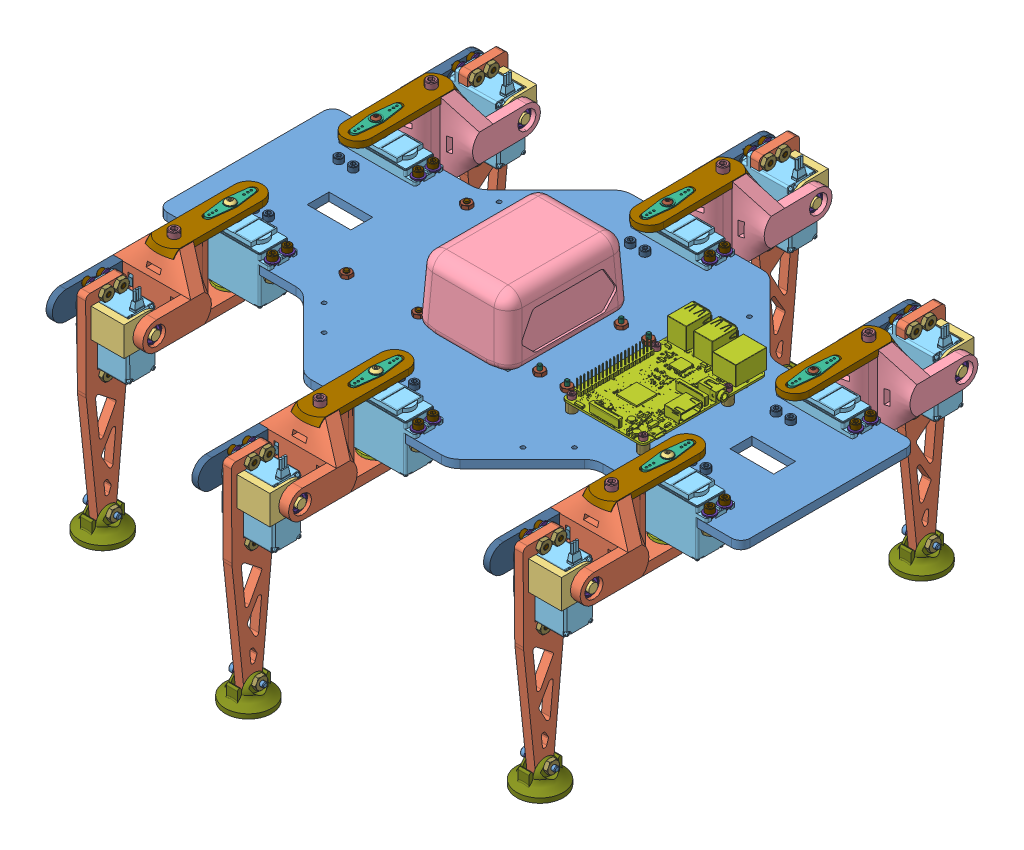
SolidWorks assembly Hexapod, configuration Défaut. Lengths in mm. (continued)
Components (placement in the parent): (continued)
- Battery-1: Battery [Défaut] at (-209.6397 14.6626 -46.247) x (-1 0 0) z (0 0 1) size (64.47 74.3 85.78)
  - MAKITA 4.0AH-1: MAKITA 4.0AH [Défaut] at (0.5853 -29.7874 85.4436) size (64.47 57.15 85.78)
  - MAKITA 4.0AH MOBILE-1: MAKITA 4.0AH MOBILE [Défaut] at (0.5853 -39.3124 91.7936) size (45.84 26.68 66.29)
- arduinoMega-1: arduinoMega [Detailed] at (-270.251 -7.6 40.62) x (0 0 -1) z (-1 0 0) size (108.32 14.5 53.3)
- raspberryPi3B-1: raspberryPi3B [Detailed] at (-112.5 6.35 40) x (0 0 -1) z (0 1 0) size (87.05 58.5 19.5)
- 12Channel PWM-1: 12Channel PWM [Default] at (-160.6 -5.6 40) x (-1 0 0) z (0 0 1) size (25.4 7.55 66.7)
- DROK_090483.stp-1: DROK_090483.stp [Default] at (-90.995 -5.6 69.895) x (-1 0 0) z (0 -1 0) size (50.02 60 18.9)
- HX-SHCS 0.138-32x0.625x0.625-N-2: HX-SHCS 0.138-32x0.625x0.625-N [HX-SHCS 0.138-32x0.625x0.625-N] at (-54.94 3.5052 69.09) x (0 -1 0) z (1 0 0) size (19.38 5.74 5.74)
- HX-SHCS 0.138-32x0.625x0.625-N-3: HX-SHCS 0.138-32x0.625x0.625-N [HX-SHCS 0.138-32x0.625x0.625-N] at (-64.94 3.5052 69.09) x (0 -1 0) z (0.5 0 0.866025) size (19.38 5.74 5.74)
- HX-SHCS 0.138-32x0.625x0.625-N-4: HX-SHCS 0.138-32x0.625x0.625-N [HX-SHCS 0.138-32x0.625x0.625-N] at (-64.94 3.5052 10.91) x (0 -1 0) z (1 0 0) size (19.38 5.74 5.74)
- HX-SHCS 0.138-32x0.625x0.625-N-5: HX-SHCS 0.138-32x0.625x0.625-N [HX-SHCS 0.138-32x0.625x0.625-N] at (-54.94 3.5052 10.91) x (0 -1 0) z (1 0 0) size (19.38 5.74 5.74)
- HX-SHCS 0.138-32x0.625x0.625-N-6: HX-SHCS 0.138-32x0.625x0.625-N [HX-SHCS 0.138-32x0.625x0.625-N] at (-214.94 3.5052 119.09) x (0 -1 0) z (1 0 0) size (19.38 5.74 5.74)
- HX-SHCS 0.138-32x0.625x0.625-N-7: HX-SHCS 0.138-32x0.625x0.625-N [HX-SHCS 0.138-32x0.625x0.625-N] at (-204.94 3.5052 119.09) x (0 -1 0) z (1 0 0) size (19.38 5.74 5.74)
- HX-SHCS 0.138-32x0.625x0.625-N-14: HX-SHCS 0.138-32x0.625x0.625-N [HX-SHCS 0.138-32x0.625x0.625-N] at (-204.94 3.5052 -39.09) x (0 -1 0) z (1 0 0) size (19.38 5.74 5.74)
- HX-SHCS 0.138-32x0.625x0.625-N-15: HX-SHCS 0.138-32x0.625x0.625-N [HX-SHCS 0.138-32x0.625x0.625-N] at (-214.94 3.5052 -39.09) x (0 -1 0) z (1 0 0) size (19.38 5.74 5.74)
- HX-SHCS 0.138-32x0.625x0.625-N-16: HX-SHCS 0.138-32x0.625x0.625-N [HX-SHCS 0.138-32x0.625x0.625-N] at (-354.94 3.5052 69.09) x (0 -1 0) z (1 0 0) size (19.38 5.74 5.74)
- HX-SHCS 0.138-32x0.625x0.625-N-17: HX-SHCS 0.138-32x0.625x0.625-N [HX-SHCS 0.138-32x0.625x0.625-N] at (-364.94 3.5052 69.09) x (0 -1 0) z (0.5 0 0.866025) size (19.38 5.74 5.74)
- HX-SHCS 0.138-32x0.625x0.625-N-18: HX-SHCS 0.138-32x0.625x0.625-N [HX-SHCS 0.138-32x0.625x0.625-N] at (-364.94 3.5052 10.91) x (0 -1 0) z (1 0 0) size (19.38 5.74 5.74)
- HX-SHCS 0.138-32x0.625x0.625-N-19: HX-SHCS 0.138-32x0.625x0.625-N [HX-SHCS 0.138-32x0.625x0.625-N] at (-354.94 3.5052 10.91) x (0 -1 0) z (1 0 0) size (19.38 5.74 5.74)
- MSHXNUT 0.138-32-D-N-60: MSHXNUT 0.138-32-D-N [MSHXNUT 0.138-32-D-N] at (-373.75 -8.4956 -15.08) x (1 0 0) z (0 -1 0) size (7.92 9.15 2.9)
- MSHXNUT 0.138-32-D-N-65: MSHXNUT 0.138-32-D-N [MSHXNUT 0.138-32-D-N] at (-373.75 -8.4956 -4.92) x (1 0 0) z (0 -1 0) size (7.92 9.15 2.9)
- MSHXNUT 0.138-32-D-N-70: MSHXNUT 0.138-32-D-N [MSHXNUT 0.138-32-D-N] at (-326.252 -8.4956 -4.92) x (0.5 0 0.866025) z (0 -1 0) size (7.92 9.15 2.9)
- MSHXNUT 0.138-32-D-N-75: MSHXNUT 0.138-32-D-N [MSHXNUT 0.138-32-D-N] at (-326.252 -8.4956 -15.08) x (0.5 0 0.866025) z (0 -1 0) size (7.92 9.15 2.9)
- MSHXNUT 0.138-32-D-N-80: MSHXNUT 0.138-32-D-N [MSHXNUT 0.138-32-D-N] at (-354.94 -13.5656 10.91) x (0 0 1) z (0 -1 0) size (7.92 9.15 2.9)
- MSHXNUT 0.138-32-D-N-85: MSHXNUT 0.138-32-D-N [MSHXNUT 0.138-32-D-N] at (-364.94 -13.5656 10.91) x (0 0 1) z (0 -1 0) size (7.92 9.15 2.9)
- MSHXNUT 0.138-32-D-N-88: MSHXNUT 0.138-32-D-N [MSHXNUT 0.138-32-D-N] at (-223.75 -8.4956 -65.08) x (1 0 0) z (0 -1 0) size (7.92 9.15 2.9)
- MSHXNUT 0.138-32-D-N-89: MSHXNUT 0.138-32-D-N [MSHXNUT 0.138-32-D-N] at (-223.75 -8.4956 -54.92) x (1 0 0) z (0 -1 0) size (7.92 9.15 2.9)
- MSHXNUT 0.138-32-D-N-90: MSHXNUT 0.138-32-D-N [MSHXNUT 0.138-32-D-N] at (-176.252 -8.4956 -54.92) x (0.5 0 0.866025) z (0 -1 0) size (7.92 9.15 2.9)
- MSHXNUT 0.138-32-D-N-91: MSHXNUT 0.138-32-D-N [MSHXNUT 0.138-32-D-N] at (-176.252 -8.4956 -65.08) x (0.5 0 0.866025) z (0 -1 0) size (7.92 9.15 2.9)
- MSHXNUT 0.138-32-D-N-92: MSHXNUT 0.138-32-D-N [MSHXNUT 0.138-32-D-N] at (-204.94 -13.5656 -39.09) x (0 0 1) z (0 -1 0) size (7.92 9.15 2.9)
- MSHXNUT 0.138-32-D-N-93: MSHXNUT 0.138-32-D-N [MSHXNUT 0.138-32-D-N] at (-214.94 -13.5656 -39.09) x (0 0 1) z (0 -1 0) size (7.92 9.15 2.9)
- MSHXNUT 0.138-32-D-N-94: MSHXNUT 0.138-32-D-N [MSHXNUT 0.138-32-D-N] at (-64.94 -13.5656 10.91) x (0 0 1) z (0 -1 0) size (7.92 9.15 2.9)
- MSHXNUT 0.138-32-D-N-95: MSHXNUT 0.138-32-D-N [MSHXNUT 0.138-32-D-N] at (-54.94 -13.5656 10.91) x (0 0 1) z (0 -1 0) size (7.92 9.15 2.9)
- MSHXNUT 0.138-32-D-N-96: MSHXNUT 0.138-32-D-N [MSHXNUT 0.138-32-D-N] at (-26.252 -8.4956 -4.92) x (0.5 0 0.866025) z (0 -1 0) size (7.92 9.15 2.9)
- MSHXNUT 0.138-32-D-N-97: MSHXNUT 0.138-32-D-N [MSHXNUT 0.138-32-D-N] at (-26.252 -8.4956 -15.08) x (0.5 0 0.866025) z (0 -1 0) size (7.92 9.15 2.9)
- MSHXNUT 0.138-32-D-N-98: MSHXNUT 0.138-32-D-N [MSHXNUT 0.138-32-D-N] at (-73.75 -8.4956 -4.92) x (1 0 0) z (0 -1 0) size (7.92 9.15 2.9)
- MSHXNUT 0.138-32-D-N-99: MSHXNUT 0.138-32-D-N [MSHXNUT 0.138-32-D-N] at (-73.75 -8.4956 -15.08) x (1 0 0) z (0 -1 0) size (7.92 9.15 2.9)
- MSHXNUT 0.138-32-D-N-100: MSHXNUT 0.138-32-D-N [MSHXNUT 0.138-32-D-N] at (-364.94 -10.67 69.09) x (0 0 -1) z (0 1 0) size (7.92 9.15 2.9)
- MSHXNUT 0.138-32-D-N-101: MSHXNUT 0.138-32-D-N [MSHXNUT 0.138-32-D-N] at (-354.94 -10.67 69.09) x (0 0 -1) z (0 1 0) size (7.92 9.15 2.9)
- MSHXNUT 0.138-32-D-N-102: MSHXNUT 0.138-32-D-N [MSHXNUT 0.138-32-D-N] at (-326.252 -5.6 84.92) x (0.5 0 -0.866025) z (0 1 0) size (7.92 9.15 2.9)
- MSHXNUT 0.138-32-D-N-103: MSHXNUT 0.138-32-D-N [MSHXNUT 0.138-32-D-N] at (-326.252 -5.6 95.08) x (0.5 0 -0.866025) z (0 1 0) size (7.92 9.15 2.9)
- MSHXNUT 0.138-32-D-N-104: MSHXNUT 0.138-32-D-N [MSHXNUT 0.138-32-D-N] at (-373.75 -5.6 84.92) x (1 0 0) z (0 1 0) size (7.92 9.15 2.9)
- MSHXNUT 0.138-32-D-N-105: MSHXNUT 0.138-32-D-N [MSHXNUT 0.138-32-D-N] at (-373.75 -5.6 95.08) x (1 0 0) z (0 1 0) size (7.92 9.15 2.9)
- MSHXNUT 0.138-32-D-N-106: MSHXNUT 0.138-32-D-N [MSHXNUT 0.138-32-D-N] at (-223.75 -5.6 145.08) x (1 0 0) z (0 1 0) size (7.92 9.15 2.9)
- MSHXNUT 0.138-32-D-N-107: MSHXNUT 0.138-32-D-N [MSHXNUT 0.138-32-D-N] at (-223.75 -5.6 134.92) x (1 0 0) z (0 1 0) size (7.92 9.15 2.9)
- MSHXNUT 0.138-32-D-N-108: MSHXNUT 0.138-32-D-N [MSHXNUT 0.138-32-D-N] at (-176.252 -5.6 134.92) x (0.5 0 -0.866025) z (0 1 0) size (7.92 9.15 2.9)
- MSHXNUT 0.138-32-D-N-109: MSHXNUT 0.138-32-D-N [MSHXNUT 0.138-32-D-N] at (-176.252 -5.6 145.08) x (0.5 0 -0.866025) z (0 1 0) size (7.92 9.15 2.9)
- MSHXNUT 0.138-32-D-N-110: MSHXNUT 0.138-32-D-N [MSHXNUT 0.138-32-D-N] at (-204.94 -10.67 119.09) x (0 0 -1) z (0 1 0) size (7.92 9.15 2.9)
- MSHXNUT 0.138-32-D-N-111: MSHXNUT 0.138-32-D-N [MSHXNUT 0.138-32-D-N] at (-214.94 -10.67 119.09) x (0 0 -1) z (0 1 0) size (7.92 9.15 2.9)
- MSHXNUT 0.138-32-D-N-112: MSHXNUT 0.138-32-D-N [MSHXNUT 0.138-32-D-N] at (-64.94 -10.67 69.09) x (0 0 -1) z (0 1 0) size (7.92 9.15 2.9)
- MSHXNUT 0.138-32-D-N-113: MSHXNUT 0.138-32-D-N [MSHXNUT 0.138-32-D-N] at (-54.94 -10.67 69.09) x (0 0 -1) z (0 1 0) size (7.92 9.15 2.9)
- MSHXNUT 0.138-32-D-N-114: MSHXNUT 0.138-32-D-N [MSHXNUT 0.138-32-D-N] at (-26.252 -5.6 84.92) x (0.5 0 -0.866025) z (0 1 0) size (7.92 9.15 2.9)
- MSHXNUT 0.138-32-D-N-115: MSHXNUT 0.138-32-D-N [MSHXNUT 0.138-32-D-N] at (-26.252 -5.6 95.08) x (0.5 0 -0.866025) z (0 1 0) size (7.92 9.15 2.9)
- MSHXNUT 0.138-32-D-N-116: MSHXNUT 0.138-32-D-N [MSHXNUT 0.138-32-D-N] at (-73.75 -5.6 84.92) x (1 0 0) z (0 1 0) size (7.92 9.15 2.9)
- MSHXNUT 0.138-32-D-N-117: MSHXNUT 0.138-32-D-N [MSHXNUT 0.138-32-D-N] at (-73.75 -5.6 95.08) x (1 0 0) z (0 1 0) size (7.92 9.15 2.9)
- HX-SHCS 0.138-32x0.5x0.5-N-20: HX-SHCS 0.138-32x0.5x0.5-N [HX-SHCS 0.138-32x0.5x0.5-N] at (-246.141 -12.6052 74.88) x (0 1 0) z (-0.5 0 -0.866025) size (16.21 5.74 5.74)
- HX-SHCS 0.138-32x0.5x0.5-N-21: HX-SHCS 0.138-32x0.5x0.5-N [HX-SHCS 0.138-32x0.5x0.5-N] at (-294.361 -12.6052 -6.36) x (0 1 0) z (1 0 0) size (16.21 5.74 5.74)
- HX-SHCS 0.138-32x0.5x0.5-N-22: HX-SHCS 0.138-32x0.5x0.5-N [HX-SHCS 0.138-32x0.5x0.5-N] at (-246.141 -12.6052 0) x (0 1 0) z (-0.5 0 -0.866025) size (16.21 5.74 5.74)
- HX-SHCS 0.138-32x0.5x0.5-N-23: HX-SHCS 0.138-32x0.5x0.5-N [HX-SHCS 0.138-32x0.5x0.5-N] at (-294.361 -12.6052 76.11) x (0 1 0) z (-1 0 0) size (16.21 5.74 5.74)
- MSHXNUT 0.112-40-D-N-106: MSHXNUT 0.112-40-D-N [MSHXNUT 0.112-40-D-N] at (-294.361 2.4892 -6.36) x (1 0 0) z (0 1 0) size (6.35 7.33 2.49)
- MSHXNUT 0.112-40-D-N-107: MSHXNUT 0.112-40-D-N [MSHXNUT 0.112-40-D-N] at (-294.361 2.4892 76.11) x (1 0 0) z (0 1 0) size (6.35 7.33 2.49)
- MSHXNUT 0.112-40-D-N-108: MSHXNUT 0.112-40-D-N [MSHXNUT 0.112-40-D-N] at (-246.141 2.4892 0) x (1 0 0) z (0 1 0) size (6.35 7.33 2.49)
- MSHXNUT 0.112-40-D-N-109: MSHXNUT 0.112-40-D-N [MSHXNUT 0.112-40-D-N] at (-246.141 2.4892 74.88) x (1 0 0) z (0 1 0) size (6.35 7.33 2.49)
- HX-SHCS 0.138-32x0.5x0.5-N-24: HX-SHCS 0.138-32x0.5x0.5-N [HX-SHCS 0.138-32x0.5x0.5-N] at (-130.81 -10.3052 13.48) x (0 1 0) z (-0.5 0 -0.866025) size (16.21 5.74 5.74)
- MSHXNUT 0.112-40-D-N-110: MSHXNUT 0.112-40-D-N [MSHXNUT 0.112-40-D-N] at (-130.81 2.4892 13.48) x (1 0 0) z (0 1 0) size (6.35 7.33 2.49)
- HX-SHCS 0.138-32x0.5x0.5-N-28: HX-SHCS 0.138-32x0.5x0.5-N [HX-SHCS 0.138-32x0.5x0.5-N] at (-94.18 -10.3052 13.48) x (0 1 0) z (-0.5 0 -0.866025) size (16.21 5.74 5.74)
- HX-SHCS 0.138-32x0.5x0.5-N-29: HX-SHCS 0.138-32x0.5x0.5-N [HX-SHCS 0.138-32x0.5x0.5-N] at (-130.81 -10.3052 66.31) x (0 1 0) z (-0.5 0 -0.866025) size (16.21 5.74 5.74)
- HX-SHCS 0.138-32x0.5x0.5-N-30: HX-SHCS 0.138-32x0.5x0.5-N [HX-SHCS 0.138-32x0.5x0.5-N] at (-94.18 -10.3052 66.31) x (0 1 0) z (-0.5 0 -0.866025) size (16.21 5.74 5.74)
- MSHXNUT 0.112-40-D-N-114: MSHXNUT 0.112-40-D-N [MSHXNUT 0.112-40-D-N] at (-94.18 2.4892 13.48) x (1 0 0) z (0 1 0) size (6.35 7.33 2.49)
- MSHXNUT 0.112-40-D-N-115: MSHXNUT 0.112-40-D-N [MSHXNUT 0.112-40-D-N] at (-130.81 2.4892 66.31) x (1 0 0) z (0 1 0) size (6.35 7.33 2.49)
- MSHXNUT 0.112-40-D-N-116: MSHXNUT 0.112-40-D-N [MSHXNUT 0.112-40-D-N] at (-94.18 2.4892 66.31) x (1 0 0) z (0 1 0) size (6.35 7.33 2.49)
- 1_4_Round_Aluminum_Standoff.step-1: 1_4_Round_Aluminum_Standoff.step [Défaut] at (-88 0 21) x (0.963282 0 -0.268492) z (0.268492 0 0.963282) size (6.34 6.36 6.34)
- HX-SHCS 0.112-40x1x0.75-N-28: HX-SHCS 0.112-40x1x0.75-N [HX-SHCS 0.112-40x1x0.75-N] at (-88 10.4948 21) x (0 -1 0) z (0.5 0 0.866025) size (28.24 4.65 4.65)
- MSHXNUT 0.112-40-D-N-117: MSHXNUT 0.112-40-D-N [MSHXNUT 0.112-40-D-N] at (-88 -8.0892 21) x (1 0 0) z (0 -1 0) size (6.35 7.33 2.49)
- 1_4_Round_Aluminum_Standoff.step-2: 1_4_Round_Aluminum_Standoff.step [Défaut] at (-137 0 21) x (0.963282 0 -0.268492) z (0.268492 0 0.963282) size (6.34 6.36 6.34)
- 1_4_Round_Aluminum_Standoff.step-3: 1_4_Round_Aluminum_Standoff.step [Défaut] at (-88 0 79) x (0.963282 0 -0.268492) z (0.268492 0 0.963282) size (6.34 6.36 6.34)
- 1_4_Round_Aluminum_Standoff.step-4: 1_4_Round_Aluminum_Standoff.step [Défaut] at (-137 0 79) x (0.963282 0 -0.268492) z (0.268492 0 0.963282) size (6.34 6.36 6.34)
- MSHXNUT 0.112-40-D-N-121: MSHXNUT 0.112-40-D-N [MSHXNUT 0.112-40-D-N] at (-137 -8.0892 21) x (1 0 0) z (0 -1 0) size (6.35 7.33 2.49)
- MSHXNUT 0.112-40-D-N-122: MSHXNUT 0.112-40-D-N [MSHXNUT 0.112-40-D-N] at (-88 -8.0892 79) x (1 0 0) z (0 -1 0) size (6.35 7.33 2.49)
- MSHXNUT 0.112-40-D-N-123: MSHXNUT 0.112-40-D-N [MSHXNUT 0.112-40-D-N] at (-137 -8.0892 79) x (1 0 0) z (0 -1 0) size (6.35 7.33 2.49)
- HX-SHCS 0.112-40x1x0.75-N-32: HX-SHCS 0.112-40x1x0.75-N [HX-SHCS 0.112-40x1x0.75-N] at (-137 10.4948 21) x (0 -1 0) z (0.5 0 0.866025) size (28.24 4.65 4.65)
- HX-SHCS 0.112-40x1x0.75-N-33: HX-SHCS 0.112-40x1x0.75-N [HX-SHCS 0.112-40x1x0.75-N] at (-88 10.4948 79) x (0 -1 0) z (0.5 0 0.866025) size (28.24 4.65 4.65)
- HX-SHCS 0.112-40x1x0.75-N-34: HX-SHCS 0.112-40x1x0.75-N [HX-SHCS 0.112-40x1x0.75-N] at (-137 10.4948 79) x (0 -1 0) z (0.5 0 0.866025) size (28.24 4.65 4.65)
- HX-SHCS 0.112-40x0.5x0.5-N-32: HX-SHCS 0.112-40x0.5x0.5-N [HX-SHCS 0.112-40x0.5x0.5-N] at (-170 -9.9448 12.05) x (0 1 0) z (-1 0 0) size (15.54 4.65 4.65)
- MSHXNUT 0.112-40-D-N-124: MSHXNUT 0.112-40-D-N [MSHXNUT 0.112-40-D-N] at (-170 2.4892 12.05) x (1 0 0) z (0 1 0) size (6.35 7.33 2.49)
- HX-SHCS 0.112-40x0.5x0.5-N-36: HX-SHCS 0.112-40x0.5x0.5-N [HX-SHCS 0.112-40x0.5x0.5-N] at (-151.2 -9.9448 12.05) x (0 1 0) z (-1 0 0) size (15.54 4.65 4.65)
- HX-SHCS 0.112-40x0.5x0.5-N-37: HX-SHCS 0.112-40x0.5x0.5-N [HX-SHCS 0.112-40x0.5x0.5-N] at (-170 -9.9448 67.95) x (0 1 0) z (-1 0 0) size (15.54 4.65 4.65)
- HX-SHCS 0.112-40x0.5x0.5-N-38: HX-SHCS 0.112-40x0.5x0.5-N [HX-SHCS 0.112-40x0.5x0.5-N] at (-151.2 -9.9448 67.95) x (0 1 0) z (-1 0 0) size (15.54 4.65 4.65)
- MSHXNUT 0.112-40-D-N-128: MSHXNUT 0.112-40-D-N [MSHXNUT 0.112-40-D-N] at (-151.2 2.4892 12.05) x (1 0 0) z (0 1 0) size (6.35 7.33 2.49)
- MSHXNUT 0.112-40-D-N-129: MSHXNUT 0.112-40-D-N [MSHXNUT 0.112-40-D-N] at (-170 2.4892 67.95) x (1 0 0) z (0 1 0) size (6.35 7.33 2.49)
- MSHXNUT 0.112-40-D-N-130: MSHXNUT 0.112-40-D-N [MSHXNUT 0.112-40-D-N] at (-151.2 2.4892 67.95) x (1 0 0) z (0 1 0) size (6.35 7.33 2.49)
Mates (geometry in assembly coordinates):
- Coincident2: coincident anti-aligned: plane of Body-1 through (-370 -5.601 0) normal (0 0 -1)
- Coincident3: coincident aligned: plane of Body-1 through (-400 0 40) normal (0 1 0)
- Coincident4: coincident aligned: plane of Body-1 through (0 0 100) normal (1 0 0)
- Coincident5: coincident anti-aligned: plane of Body-1 through (-400 0 40) normal (0 1 0); plane of Assembly_Leg_V4-1/hs-422-3 through (-50.001 0 -0.094) normal (0 -1 0)
- Concentric3: concentric anti-aligned: cylinder of Body-1 through (-73.75 0 -15.08) axis (0 -1 0) radius 1.45; cylinder of Assembly_Leg_V4-1/hs-422-3 through (-73.75 -26.67 -15.08) axis (0 1 0) radius 2.1844
- Concentric6: concentric aligned: cylinder of Body-1 through (-373.75 -5.601 -4.92) axis (0 1 0) radius 1.45; cylinder of Assembly_Leg_V4-2/hs-422-3 through (-373.75 -26.67 -4.92) axis (0 1 0) radius 2.1844
- Parallel4: parallel anti-aligned: plane of Body-1 through (-370 -5.601 0) normal (0 0 -1); plane of Assembly_Leg_V4-2/hs-422-3 through (-350.001 -5.969 -0.094) normal (0 0 1)
- Coincident9: coincident anti-aligned: plane of Body-1 through (-400 0 40) normal (0 1 0); plane of Assembly_Leg_V4-2/hs-422-3 through (-350.001 0 -0.094) normal (0 -1 0)
- Coincident10: coincident anti-aligned: plane of Body-1 through (-400 0 40) normal (0 1 0); plane of Assembly_Leg_V4-3/hs-422-3 through (-200.001 0 -50.094) normal (0 -1 0)
- Concentric7: concentric anti-aligned: cylinder of Body-1 through (-223.75 0 -54.92) axis (0 -1 0) radius 1.45; cylinder of Assembly_Leg_V4-3/hs-422-3 through (-223.75 -26.67 -54.92) axis (0 1 0) radius 2.1844
- Parallel5: parallel anti-aligned: plane of Body-1 through (-220 -5.6 -50) normal (0 0 -1); plane of Assembly_Leg_V4-3/hs-422-3 through (-200.001 -5.969 -50.094) normal (0 0 1)
- Parallel6: parallel anti-aligned: plane of Body-1 through (-70 -5.6 0) normal (0 0 -1); plane of Assembly_Leg_V4-1/hs-422-3 through (-50.001 -5.969 -0.094) normal (0 0 1)
- Coincident11: coincident anti-aligned: plane of Body-1 through (-400 0 40) normal (0 1 0); plane of Assembly_Leg_V4_Mirror-1/hs-422-3 through (-350.001 0 99.906) normal (0 -1 0)
- Concentric8: concentric aligned: cylinder of Body-1 through (-373.75 -5.601 95.08) axis (0 1 0) radius 1.45; cylinder of Assembly_Leg_V4_Mirror-1/hs-422-3 through (-373.75 -26.67 95.08) axis (0 1 0) radius 2.1844
- Parallel7: parallel anti-aligned: plane of Body-1 through (-370 -5.601 80) normal (0 0 1); plane of Assembly_Leg_V4_Mirror-1/hs-422-3 through (-350.001 -5.969 80.094) normal (0 0 -1)
- Coincident13: coincident anti-aligned: plane of Body-1 through (-400 0 40) normal (0 1 0); plane of Assembly_Leg_V4_Mirror-2/hs-422-3 through (-50.001 0 99.906) normal (0 -1 0)
- Concentric9: concentric anti-aligned: cylinder of Body-1 through (-73.75 0 95.08) axis (0 -1 0) radius 1.45; cylinder of Assembly_Leg_V4_Mirror-2/hs-422-3 through (-73.75 -26.67 95.08) axis (0 1 0) radius 2.1844
- Parallel8: parallel anti-aligned: plane of Body-1 through (-70 -5.6 80) normal (0 0 1); plane of Assembly_Leg_V4_Mirror-2/hs-422-3 through (-50.001 -5.969 80.094) normal (0 0 -1)
- Coincident15: coincident anti-aligned: plane of Body-1 through (-400 0 40) normal (0 1 0); plane of Assembly_Leg_V4_Mirror-3/hs-422-3 through (-200.001 0 149.906) normal (0 -1 0)
- Concentric10: concentric anti-aligned: cylinder of Body-1 through (-223.75 0 145.08) axis (0 -1 0) radius 1.45; cylinder of Assembly_Leg_V4_Mirror-3/hs-422-3 through (-223.75 -26.67 145.08) axis (0 1 0) radius 2.1844
- Parallel9: parallel anti-aligned: plane of Body-1 through (-220 -5.6 130) normal (0 0 1); plane of Assembly_Leg_V4_Mirror-3/hs-422-3 through (-200.001 -5.969 130.094) normal (0 0 -1)
- Coïncidente1: coincident anti-aligned: plane of Body-1 through (-400 0 40) normal (0 1 0); plane of Batterie-1/MAKITA 4.0AH-1 through (-210.225 0 39.1966) normal (0 -1 0)
- Coïncidente2: coincident anti-aligned: plane of arduinoMega-1 through (-270.251 -5.6 40.62) normal (0 1 0); plane of Body-1 through (-400 -5.6 40) normal (0 -1 0)
- Coïncidente4: coincident anti-aligned: plane of Body-1 through (-400 -5.6 40) normal (0 -1 0); plane of 12Channel PWM-1 through (-170 -5.6 12.05) normal (0 1 0)
- Coïncidente5: coincident anti-aligned: plane of Body-1 through (-400 -5.6 40) normal (0 -1 0); plane of DROK_090483.stp-1 through (-112.495 -5.6 39.895) normal (0 1 0)
- Parallèle4: parallel aligned: plane of Body-1 through (0 0 100) normal (1 0 0); plane of 12Channel PWM-1 through (-147.9 -7.1 12.05) normal (1 0 0)
- Concentric13: concentric aligned: cylinder of Body-1 through (-170 0 67.95) axis (0 -1 0) radius 1.25; cylinder of 12Channel PWM-1 through (-170 -2.0645 67.95) axis (0 -1 0) radius 1.25
- Concentric15: concentric aligned: cylinder of Body-1 through (-137 -5.6 21) axis (0 1 0) radius 1.375; cylinder of raspberryPi3B-1 through (-137 6.35 21) axis (0 1 0) radius 1.375
- Concentric16: concentric aligned: cylinder of Body-1 through (-88 -5.6 79) axis (0 1 0) radius 1.375; cylinder of raspberryPi3B-1 through (-88 6.35 79) axis (0 1 0) radius 1.375
- Coincident17: coincident anti-aligned: plane of Body-1 through (-232.45 0 2.16) normal (1 0 0); plane of Batterie-1/MAKITA 4.0AH MOBILE-1 through (-232.45 53.975 45.5466) normal (-1 0 0)
- Coincident18: coincident anti-aligned: plane of Body-1 through (-232.45 0 77.85) normal (0 0 -1); plane of Batterie-1/MAKITA 4.0AH MOBILE-1 through (-192.7625 -22.225 77.85) normal (0 0 1)
- Concentric17: concentric anti-aligned: circle of Body-1; circle of DROK_090483.stp-1
- Concentric18: concentric aligned: cylinder of Body-1 through (-94.18 0 66.31) axis (0 -1 0) radius 1.45; cylinder of DROK_090483.stp-1 through (-94.18 -5.6 66.31) axis (0 -1 0) radius 1.585
- Concentric19: concentric aligned: cylinder of Body-1 through (-246.141 0 0) axis (0 -1 0) radius 1.6; circle of arduinoMega-1
- Concentric22: concentric aligned: cylinder of Body-1 through (-294.361 0 76.11) axis (0 -1 0) radius 1.6; cylinder of arduinoMega-1 through (-294.361 -7.6 76.11) axis (0 -1 0) radius 1.6
- Concentric23: concentric anti-aligned: cylinder of Body-1 through (-54.94 0 69.09) axis (0 -1 0) radius 1.45; cylinder of HX-SHCS 0.138-32x0.625x0.625-N-2 through (-54.94 35.2552 69.09) axis (0 1 0) radius 1.7526
- Concentric24: concentric anti-aligned: cylinder of Body-1 through (-64.94 0 69.09) axis (0 -1 0) radius 1.45; cylinder of HX-SHCS 0.138-32x0.625x0.625-N-3 through (-64.94 35.2552 69.09) axis (0 1 0) radius 1.7526
- Coincident19: coincident anti-aligned: plane of Body-1 through (-400 0 40) normal (0 1 0); plane of HX-SHCS 0.138-32x0.625x0.625-N-2 through (-54.94 0 66.2198) normal (0 -1 0)
- Coincident20: coincident anti-aligned: plane of Body-1 through (-400 0 40) normal (0 1 0); plane of HX-SHCS 0.138-32x0.625x0.625-N-3 through (-62.4543 0 67.6549) normal (0 -1 0)
- Parallel10: parallel aligned: plane of Body-1 through (0 0 100) normal (1 0 0); plane of HX-SHCS 0.138-32x0.625x0.625-N-3 through (-66.3243 1.8796 69.8892) normal (1 0 0)
- Parallel11: parallel aligned: plane of Body-1 through (0 0 100) normal (1 0 0); plane of HX-SHCS 0.138-32x0.625x0.625-N-2 through (-56.3243 1.8796 68.2908) normal (1 0 0)
- Concentric25: concentric anti-aligned: cylinder of Body-1 through (-64.94 0 10.91) axis (0 -1 0) radius 1.45; cylinder of HX-SHCS 0.138-32x0.625x0.625-N-4 through (-64.94 35.2552 10.91) axis (0 1 0) radius 1.7526
- Concentric26: concentric anti-aligned: cylinder of Body-1 through (-54.94 0 10.91) axis (0 -1 0) radius 1.45; cylinder of HX-SHCS 0.138-32x0.625x0.625-N-5 through (-54.94 35.2552 10.91) axis (0 1 0) radius 1.7526
- Coincident23: coincident anti-aligned: plane of Body-1 through (-400 0 40) normal (0 1 0); plane of HX-SHCS 0.138-32x0.625x0.625-N-5 through (-54.94 0 8.0398) normal (0 -1 0)
- Coincident24: coincident anti-aligned: plane of Body-1 through (-400 0 40) normal (0 1 0); plane of HX-SHCS 0.138-32x0.625x0.625-N-4 through (-64.94 0 8.0398) normal (0 -1 0)
- Parallel12: parallel aligned: plane of Body-1 through (0 0 100) normal (1 0 0); plane of HX-SHCS 0.138-32x0.625x0.625-N-5 through (-56.3243 1.8796 10.1108) normal (1 0 0)
- Parallel13: parallel aligned: plane of Body-1 through (0 0 100) normal (1 0 0); plane of HX-SHCS 0.138-32x0.625x0.625-N-4 through (-66.3243 1.8796 10.1108) normal (1 0 0)
- Concentric27: concentric anti-aligned: cylinder of Body-1 through (-214.94 0 -39.09) axis (0 -1 0) radius 1.45; cylinder of HX-SHCS 0.138-32x0.625x0.625-N-13 through (-214.94 40.2807 -39.09) axis (0 1 0) radius 1.7526
- Concentric29: concentric anti-aligned: cylinder of Body-1 through (-204.94 0 119.09) axis (0 -1 0) radius 1.45; cylinder of HX-SHCS 0.138-32x0.625x0.625-N-7 through (-204.94 35.2552 119.09) axis (0 1 0) radius 1.7526
- Concentric30: concentric anti-aligned: cylinder of Body-1 through (-214.94 0 119.09) axis (0 -1 0) radius 1.45; cylinder of HX-SHCS 0.138-32x0.625x0.625-N-6 through (-214.94 35.2552 119.09) axis (0 1 0) radius 1.7526
- Coincident27: coincident anti-aligned: plane of Body-1 through (-400 0 40) normal (0 1 0); plane of HX-SHCS 0.138-32x0.625x0.625-N-7 through (-204.94 0 116.2198) normal (0 -1 0)
- Coincident28: coincident anti-aligned: plane of Body-1 through (-400 0 40) normal (0 1 0); plane of HX-SHCS 0.138-32x0.625x0.625-N-6 through (-214.94 0 116.2198) normal (0 -1 0)
- Parallel14: parallel aligned: plane of Body-1 through (0 0 100) normal (1 0 0); plane of HX-SHCS 0.138-32x0.625x0.625-N-6 through (-216.3243 1.8796 118.2908) normal (1 0 0)
- Parallel15: parallel aligned: plane of Body-1 through (0 0 100) normal (1 0 0); plane of HX-SHCS 0.138-32x0.625x0.625-N-7 through (-206.3243 1.8796 118.2908) normal (1 0 0)
- Concentric31: concentric anti-aligned: cylinder of Body-1 through (-214.94 0 -39.09) axis (0 -1 0) radius 1.45; cylinder of HX-SHCS 0.138-32x0.625x0.625-N-15 through (-214.94 35.2552 -39.09) axis (0 1 0) radius 1.7526
- Concentric32: concentric anti-aligned: cylinder of Body-1 through (-204.94 0 -39.09) axis (0 -1 0) radius 1.45; cylinder of HX-SHCS 0.138-32x0.625x0.625-N-14 through (-204.94 35.2552 -39.09) axis (0 1 0) radius 1.7526
- Coincident31: coincident anti-aligned: plane of Body-1 through (-400 0 40) normal (0 1 0); plane of HX-SHCS 0.138-32x0.625x0.625-N-15 through (-214.94 0 -41.9602) normal (0 -1 0)
- Coincident32: coincident anti-aligned: plane of Body-1 through (-400 0 40) normal (0 1 0); plane of HX-SHCS 0.138-32x0.625x0.625-N-14 through (-204.94 0 -41.9602) normal (0 -1 0)
- Parallel16: parallel anti-aligned: plane of Body-1 through (0 0 100) normal (1 0 0); plane of HX-SHCS 0.138-32x0.625x0.625-N-15 through (-213.5557 1.8796 -38.2908) normal (-1 0 0)
- Parallel17: parallel anti-aligned: plane of Body-1 through (0 0 100) normal (1 0 0); plane of HX-SHCS 0.138-32x0.625x0.625-N-14 through (-203.5557 1.8796 -38.2908) normal (-1 0 0)
- Concentric33: concentric aligned: cylinder of Body-1 through (-364.94 -5.601 69.09) axis (0 1 0) radius 1.45; cylinder of HX-SHCS 0.138-32x0.625x0.625-N-17 through (-364.94 35.2552 69.09) axis (0 1 0) radius 1.7526
- Concentric34: concentric aligned: circle of Body-1; cylinder of HX-SHCS 0.138-32x0.625x0.625-N-16 through (-354.94 35.2552 69.09) axis (0 1 0) radius 1.7526
- Concentric35: concentric aligned: cylinder of Body-1 through (-364.94 -5.601 10.91) axis (0 1 0) radius 1.45; cylinder of HX-SHCS 0.138-32x0.625x0.625-N-18 through (-364.94 35.2552 10.91) axis (0 1 0) radius 1.7526
- Concentric36: concentric aligned: cylinder of Body-1 through (-354.94 -5.601 10.91) axis (0 1 0) radius 1.45; cylinder of HX-SHCS 0.138-32x0.625x0.625-N-19 through (-354.94 35.2552 10.91) axis (0 1 0) radius 1.7526
- Coincident35: coincident anti-aligned: plane of Body-1 through (-400 0 40) normal (0 1 0); plane of HX-SHCS 0.138-32x0.625x0.625-N-18 through (-364.94 0 8.0398) normal (0 -1 0)
- Coincident36: coincident anti-aligned: plane of Body-1 through (-400 0 40) normal (0 1 0); plane of HX-SHCS 0.138-32x0.625x0.625-N-19 through (-354.94 0 8.0398) normal (0 -1 0)
- Coincident37: coincident anti-aligned: plane of Body-1 through (-400 0 40) normal (0 1 0); plane of HX-SHCS 0.138-32x0.625x0.625-N-17 through (-362.4543 0 67.6549) normal (0 -1 0)
- Coincident38: coincident anti-aligned: plane of Body-1 through (-400 0 40) normal (0 1 0); plane of HX-SHCS 0.138-32x0.625x0.625-N-16 through (-354.94 0 66.2198) normal (0 -1 0)
- Parallel18: parallel anti-aligned: plane of Body-1 through (0 0 100) normal (1 0 0); plane of HX-SHCS 0.138-32x0.625x0.625-N-19 through (-353.5557 1.8796 11.7092) normal (-1 0 0)
- Parallel19: parallel anti-aligned: plane of Body-1 through (0 0 100) normal (1 0 0); plane of HX-SHCS 0.138-32x0.625x0.625-N-18 through (-363.5557 1.8796 11.7092) normal (-1 0 0)
- Parallel20: parallel anti-aligned: plane of Body-1 through (0 0 100) normal (1 0 0); plane of HX-SHCS 0.138-32x0.625x0.625-N-16 through (-353.5557 1.8796 69.8892) normal (-1 0 0)
- Parallel21: parallel anti-aligned: plane of Body-1 through (0 0 100) normal (1 0 0); plane of HX-SHCS 0.138-32x0.625x0.625-N-17 through (-363.5557 1.8796 68.2908) normal (-1 0 0)
- Concentric37: concentric anti-aligned: cylinder of Leg-2/socket_1_2_6-32_with_washer-7/HX-SHCS 0.138-32x0.5x0.5-N-1 through (-373.75 38.5826 -15.08) axis (0 1 0) radius 1.7526; circle of MSHXNUT 0.138-32-D-N-1
- Coincident40: coincident anti-aligned: plane of Body-1 through (-400 -5.6 40) normal (0 -1 0); plane of MSHXNUT 0.138-32-D-N-60 through (-381.6748 -5.6 -15.08) normal (0 1 0)
- Parallel22: parallel aligned: plane of Leg-2/hs-422-3 through (-369.94 -5.969 -0.094) normal (-1 0 0); plane of MSHXNUT 0.138-32-D-N-60 through (-377.7124 -5.6 -12.7923) normal (-1 0 0)
- Concentric38: concentric anti-aligned: cylinder of Leg-2/socket_1_2_6-32_with_washer-5/HX-SHCS 0.138-32x0.5x0.5-N-1 through (-373.75 38.5826 -4.92) axis (0 1 0) radius 1.7526; circle of MSHXNUT 0.138-32-D-N-2
- Parallel23: parallel aligned: plane of Leg-2/hs-422-3 through (-369.94 -5.969 -0.094) normal (-1 0 0); plane of MSHXNUT 0.138-32-D-N-65 through (-377.7124 -5.6 -2.6323) normal (-1 0 0)
- Coincident44: coincident anti-aligned: plane of Body-1 through (-400 -5.6 40) normal (0 -1 0); plane of MSHXNUT 0.138-32-D-N-65 through (-381.6748 -5.6 -4.92) normal (0 1 0)
- Coincident45: coincident anti-aligned: cylinder of Leg-2/socket_1_2_6-32_with_washer-8/HX-SHCS 0.138-32x0.5x0.5-N-1 through (-326.252 38.5826 -4.92) axis (0 1 0) radius 1.7526; circle of MSHXNUT 0.138-32-D-N-3
- Concentric40: concentric anti-aligned: cylinder of Leg-2/socket_1_2_6-32_with_washer-6/HX-SHCS 0.138-32x0.5x0.5-N-1 through (-326.252 38.5826 -15.08) axis (0 1 0) radius 1.7526; circle of MSHXNUT 0.138-32-D-N-4
- Coincident47: coincident anti-aligned: plane of Body-1 through (-400 -5.6 40) normal (0 -1 0); plane of MSHXNUT 0.138-32-D-N-75 through (-330.2144 -5.6 -21.9431) normal (0 1 0)
- Coincident48: coincident anti-aligned: plane of Body-1 through (-400 -5.6 40) normal (0 -1 0); plane of MSHXNUT 0.138-32-D-N-70 through (-330.2144 -5.6 -11.7831) normal (0 1 0)
- Parallel24: parallel aligned: plane of Leg-2/hs-422-3 through (-330.062 -5.969 -0.094) normal (1 0 0); plane of MSHXNUT 0.138-32-D-N-75 through (-322.2896 -5.6 -17.3677) normal (1 0 0)
- Parallel25: parallel aligned: plane of Leg-2/hs-422-3 through (-330.062 -5.969 -0.094) normal (1 0 0); plane of MSHXNUT 0.138-32-D-N-70 through (-322.2896 -5.6 -7.2077) normal (1 0 0)
- Concentric41: concentric anti-aligned: cylinder of HX-SHCS 0.138-32x0.625x0.625-N-19 through (-354.94 35.2552 10.91) axis (0 1 0) radius 1.7526; circle of MSHXNUT 0.138-32-D-N-5
- Concentric42: concentric anti-aligned: cylinder of HX-SHCS 0.138-32x0.625x0.625-N-18 through (-364.94 35.2552 10.91) axis (0 1 0) radius 1.7526; circle of MSHXNUT 0.138-32-D-N-6
- Coincident53: coincident anti-aligned: plane of Leg-2/Bearing_mount_leg-1 through (-370.288 -10.67 15) normal (0 -1 0); plane of MSHXNUT 0.138-32-D-N-85 through (-364.94 -10.67 2.9852) normal (0 1 0)
- Coincident54: coincident anti-aligned: plane of Leg-2/Bearing_mount_leg-1 through (-370.288 -10.67 15) normal (0 -1 0); plane of MSHXNUT 0.138-32-D-N-80 through (-354.94 -10.67 2.9852) normal (0 1 0)
- Parallel26: parallel aligned: plane of Leg-2/Bearing_mount_leg-1 through (-370.288 -26.67 5) normal (0 0 1); plane of MSHXNUT 0.138-32-D-N-80 through (-357.2277 -10.67 14.8724) normal (0 0 1)
- Parallel27: parallel aligned: plane of Leg-2/Bearing_mount_leg-1 through (-370.288 -26.67 5) normal (0 0 1); plane of MSHXNUT 0.138-32-D-N-85 through (-367.2277 -10.67 14.8724) normal (0 0 1)
- Concentric43: concentric aligned: cylinder of arduinoMega-1 through (-246.141 -7.6 74.88) axis (0 -1 0) radius 1.6; cylinder of HX-SHCS 0.138-32x0.5x0.5-N-20 through (-246.141 -44.3552 74.88) axis (0 -1 0) radius 1.7526
- Concentric44: concentric aligned: cylinder of arduinoMega-1 through (-294.361 -7.6 76.11) axis (0 -1 0) radius 1.6; cylinder of HX-SHCS 0.138-32x0.5x0.5-N-23 through (-294.361 -44.3552 76.11) axis (0 -1 0) radius 1.7526
- Concentric45: concentric aligned: cylinder of arduinoMega-1 through (-294.361 -7.6 -6.36) axis (0 -1 0) radius 1.6; cylinder of HX-SHCS 0.138-32x0.5x0.5-N-21 through (-294.361 -44.3552 -6.36) axis (0 -1 0) radius 1.7526
- Concentric46: concentric aligned: cylinder of arduinoMega-1 through (-246.141 -7.6 0) axis (0 -1 0) radius 1.6; cylinder of HX-SHCS 0.138-32x0.5x0.5-N-22 through (-246.141 -44.3552 0) axis (0 -1 0) radius 1.7526
- Coincident58: coincident anti-aligned: plane of arduinoMega-1 through (-270.251 -9.1 40.62) normal (0 -1 0); plane of HX-SHCS 0.138-32x0.5x0.5-N-20 through (-243.6553 -9.1 73.4449) normal (0 1 0)
- Coincident59: coincident anti-aligned: plane of arduinoMega-1 through (-270.251 -9.1 40.62) normal (0 -1 0); plane of HX-SHCS 0.138-32x0.5x0.5-N-22 through (-243.6553 -9.1 -1.4351) normal (0 1 0)
- Coincident60: coincident anti-aligned: plane of arduinoMega-1 through (-270.251 -9.1 40.62) normal (0 -1 0); plane of HX-SHCS 0.138-32x0.5x0.5-N-23 through (-294.361 -9.1 73.2398) normal (0 1 0)
- Coincident61: coincident anti-aligned: plane of arduinoMega-1 through (-270.251 -9.1 40.62) normal (0 -1 0); plane of HX-SHCS 0.138-32x0.5x0.5-N-21 through (-294.361 -9.1 -3.4898) normal (0 1 0)
- Concentric47: concentric anti-aligned: cylinder of HX-SHCS 0.138-32x0.5x0.5-N-21 through (-294.361 -44.3552 -6.36) axis (0 -1 0) radius 1.7526; circle of MSHXNUT 0.112-40-S-N-2
- Concentric48: concentric anti-aligned: cylinder of HX-SHCS 0.138-32x0.5x0.5-N-23 through (-294.361 -44.3552 76.11) axis (0 -1 0) radius 1.7526; circle of MSHXNUT 0.112-40-S-N-3
- Concentric49: concentric anti-aligned: cylinder of HX-SHCS 0.138-32x0.5x0.5-N-22 through (-246.141 -44.3552 0) axis (0 -1 0) radius 1.7526; circle of MSHXNUT 0.112-40-S-N-4
- Concentric50: concentric anti-aligned: cylinder of HX-SHCS 0.138-32x0.5x0.5-N-20 through (-246.141 -44.3552 74.88) axis (0 -1 0) radius 1.7526; circle of MSHXNUT 0.112-40-S-N-5
- Coincident62: coincident anti-aligned: plane of Body-1 through (-400 0 40) normal (0 1 0); plane of MSHXNUT 0.112-40-D-N-109 through (-252.491 0 74.88) normal (0 -1 0)
- Coincident63: coincident anti-aligned: plane of Body-1 through (-400 0 40) normal (0 1 0); plane of MSHXNUT 0.112-40-D-N-108 through (-252.491 0 0) normal (0 -1 0)
- Coincident64: coincident anti-aligned: plane of Body-1 through (-400 0 40) normal (0 1 0); plane of MSHXNUT 0.112-40-D-N-107 through (-300.711 0 76.11) normal (0 -1 0)
- Coincident65: coincident anti-aligned: plane of Body-1 through (-400 0 40) normal (0 1 0); plane of MSHXNUT 0.112-40-D-N-106 through (-300.711 0 -6.36) normal (0 -1 0)
- Parallel28: parallel anti-aligned: plane of Body-1 through (-400 0 40) normal (-1 0 0); plane of MSHXNUT 0.112-40-D-N-107 through (-291.186 0 74.2769) normal (1 0 0)
- Parallel30: parallel aligned: plane of Body-1 through (-400 0 40) normal (-1 0 0); plane of MSHXNUT 0.112-40-D-N-106 through (-297.536 0 -8.1931) normal (-1 0 0)
- Parallel31: parallel aligned: plane of Body-1 through (-400 0 40) normal (-1 0 0); plane of MSHXNUT 0.112-40-D-N-108 through (-249.316 0 -1.8331) normal (-1 0 0)
- Parallel32: parallel aligned: plane of Body-1 through (-400 0 40) normal (-1 0 0); plane of MSHXNUT 0.112-40-D-N-109 through (-249.316 0 73.0469) normal (-1 0 0)
- Parallel33: parallel aligned: plane of arduinoMega-1 through (-296.901 -9.1 90.11) normal (-1 0 0); plane of HX-SHCS 0.138-32x0.5x0.5-N-23 through (-292.9767 -10.9796 75.3108) normal (-1 0 0)
- Parallel34: parallel aligned: plane of arduinoMega-1 through (-296.901 -9.1 90.11) normal (-1 0 0); plane of HX-SHCS 0.138-32x0.5x0.5-N-20 through (-244.7567 -10.9796 74.0808) normal (-1 0 0)
- Parallel35: parallel aligned: plane of arduinoMega-1 through (-296.901 -9.1 90.11) normal (-1 0 0); plane of HX-SHCS 0.138-32x0.5x0.5-N-22 through (-244.7567 -10.9796 -0.7992) normal (-1 0 0)
- Parallel36: parallel aligned: plane of arduinoMega-1 through (-296.901 -9.1 90.11) normal (-1 0 0); plane of HX-SHCS 0.138-32x0.5x0.5-N-21 through (-292.9767 -10.9796 -7.1592) normal (-1 0 0)
- Concentric51: concentric aligned: cylinder of DROK_090483.stp-1 through (-130.81 -5.6 13.48) axis (0 -1 0) radius 1.585; cylinder of HX-SHCS 0.138-32x0.5x0.5-N-24 through (-130.81 -42.0552 13.48) axis (0 -1 0) radius 1.7526
- Coincident74: coincident anti-aligned: plane of DROK_090483.stp-1 through (-112.495 -6.8 39.895) normal (0 -1 0); plane of HX-SHCS 0.138-32x0.5x0.5-N-24 through (-128.3243 -6.8 12.0449) normal (0 1 0)
- Parallel37: parallel aligned: plane of DROK_090483.stp-1 through (-133.995 -5.6 69.895) normal (-1 0 0); plane of HX-SHCS 0.138-32x0.5x0.5-N-24 through (-129.4257 -8.6796 12.6808) normal (-1 0 0)
- Concentric52: concentric anti-aligned: cylinder of HX-SHCS 0.138-32x0.5x0.5-N-24 through (-130.81 -42.0552 13.48) axis (0 -1 0) radius 1.7526; circle of MSHXNUT 0.112-40-S-N-6
- Coincident76: coincident anti-aligned: plane of Body-1 through (-400 0 40) normal (0 1 0); plane of MSHXNUT 0.112-40-D-N-110 through (-137.16 0 13.48) normal (0 -1 0)
- Parallel38: parallel anti-aligned: plane of Body-1 through (0 0 100) normal (1 0 0); plane of MSHXNUT 0.112-40-D-N-110 through (-133.985 0 11.6469) normal (-1 0 0)
- Concentric53: concentric anti-aligned: cylinder of Body-1 through (-88 -5.6 21) axis (0 1 0) radius 1.375; cylinder of 1_4_Round_Aluminum_Standoff.step-1 through (-88 6.35 21) axis (0 -1 0) radius 3.1712
- Coincident78: coincident anti-aligned: plane of Body-1 through (-400 0 40) normal (0 1 0); plane of 1_4_Round_Aluminum_Standoff.step-1 through (-88 0 21) normal (0 -1 0)
- Coincident79: coincident anti-aligned: plane of raspberryPi3B-1 through (-112.5 6.35 40) normal (0 -1 0); plane of 1_4_Round_Aluminum_Standoff.step-1 through (-88 6.35 21) normal (0 1 0)
- Concentric54: concentric aligned: cylinder of raspberryPi3B-1 through (-88 6.35 21) axis (0 1 0) radius 1.375; cylinder of HX-SHCS 0.112-40x1x0.75-N-28 through (-88 42.2448 21) axis (0 1 0) radius 1.4224
- Coincident80: coincident anti-aligned: plane of raspberryPi3B-1 through (-112.5 7.65 40) normal (0 1 0); plane of HX-SHCS 0.112-40x1x0.75-N-28 through (-85.9873 7.65 19.8379) normal (0 -1 0)
- Parallel39: parallel aligned: plane of raspberryPi3B-1 through (-84.5 7.65 82.5) normal (1 0 0); plane of HX-SHCS 0.112-40x1x0.75-N-28 through (-89.1938 9.1994 21.6892) normal (1 0 0)
- Concentric55: concentric anti-aligned: cylinder of HX-SHCS 0.112-40x1x0.75-N-28 through (-88 42.2448 21) axis (0 1 0) radius 1.4224; circle of MSHXNUT 0.112-40-D-N-3
- Coincident83: coincident anti-aligned: plane of Body-1 through (-400 -5.6 40) normal (0 -1 0); plane of MSHXNUT 0.112-40-D-N-117 through (-94.35 -5.6 21) normal (0 1 0)
- Parallel40: parallel aligned: plane of Body-1 through (0 0 100) normal (1 0 0); plane of MSHXNUT 0.112-40-D-N-117 through (-84.825 -5.6 22.8331) normal (1 0 0)
- Concentric56: concentric aligned: cylinder of 12Channel PWM-1 through (-170 -2.0645 12.05) axis (0 -1 0) radius 1.25; cylinder of HX-SHCS 0.112-40x0.5x0.5-N-32 through (-170 -41.6948 12.05) axis (0 -1 0) radius 1.4224
- Coincident85: coincident anti-aligned: plane of 12Channel PWM-1 through (-170 -7.1 12.05) normal (0 -1 0); plane of HX-SHCS 0.112-40x0.5x0.5-N-32 through (-170 -7.1 9.7259) normal (0 1 0)
- Parallel41: parallel aligned: plane of 12Channel PWM-1 through (-147.9 -7.1 12.05) normal (1 0 0); plane of HX-SHCS 0.112-40x0.5x0.5-N-32 through (-171.1938 -8.6494 12.7392) normal (1 0 0)
- Concentric57: concentric anti-aligned: cylinder of HX-SHCS 0.112-40x0.5x0.5-N-32 through (-170 -41.6948 12.05) axis (0 -1 0) radius 1.4224; circle of MSHXNUT 0.112-40-D-N-68
- Coincident88: coincident anti-aligned: plane of Body-1 through (-400 0 40) normal (0 1 0); plane of MSHXNUT 0.112-40-D-N-124 through (-176.35 0 12.05) normal (0 -1 0)
- Parallel42: parallel aligned: plane of Body-1 through (0 0 100) normal (1 0 0); plane of MSHXNUT 0.112-40-D-N-124 through (-166.825 0 10.2169) normal (1 0 0)
